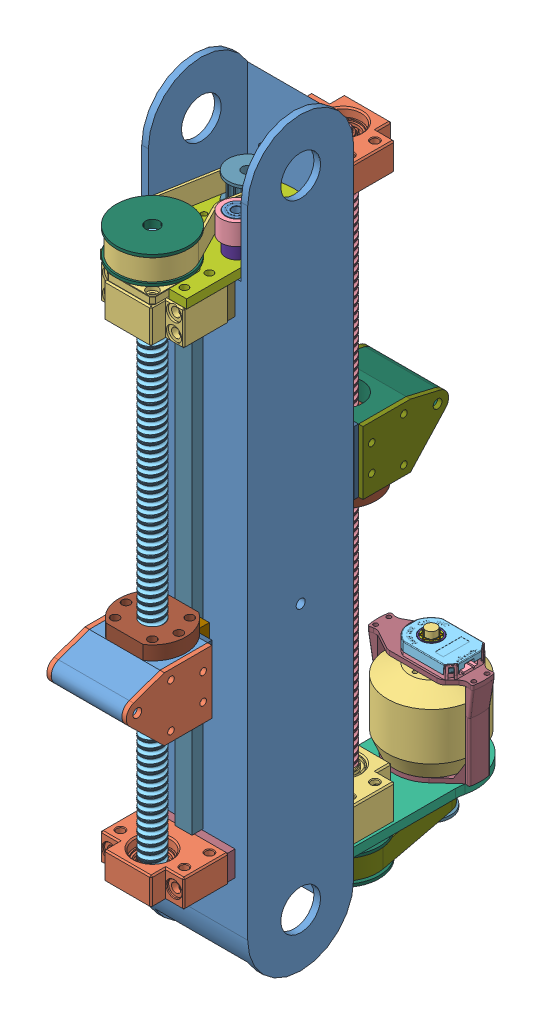
SolidWorks assembly Shoulder, configuration Default. Lengths in mm.
Overall size (98.94 533.4 280.38).
79 component instances, 40 part files, 66 mates.
Components (placement in the parent):
- Box^Shoulder-1: Box^Shoulder [Default] at origin size (76.2 533.4 76.2) (virtual)
- BF12-1: BF12 [Default] at (0 614.1315 -46.7041) x (1 0 0) z (0 1 0) size (60 43 20)
- BK12-1: BK12 [Default] at (0 212.1315 -46.7041) x (-1 0 0) z (0 -1 0) size (60 46.94 35.34)
- SFU1605-450-1: SFU1605-450 [1605-400] at (0 171.1315 -71.7041) x (1 0 0) z (0 -1 0) size (16.52 16.22 450)
- BK12-2: BK12 [Default] at (0 582.269 40.2909) x (-1 0 0) z (0 1 0) size (60 46.94 35.34)
- BF12-2: BF12 [Default] at (0 230.269 40.2909) x (-1 0 0) z (0 1 0) size (60 43 20)
- SFU1605-400-3: SFU1605-400 [1605-400] at (0 623.269 65.2909) x (-1 0 0) z (0 1 0) size (16.52 16.22 400)
- J3Plate^Shoulder-1: J3Plate^Shoulder [Default] at origin size (65 6.35 120.35) (virtual)
- J2Plate^Shoulder-1: J2Plate^Shoulder [Default] at origin size (65 6.35 125.74) (virtual)
- J3MGN12R-1: J3MGN12R [Default] at origin size (12 379.5 8)
- J3MGN12C-1: J3MGN12C [Default] at (0 433.1293 -49.3066) x (1 0 0) z (0 1 0) size (27 10 45.5)
- CarriagePlate^Shoulder-1: CarriagePlate^Shoulder [Default] at (0 67.1524 -3.2066) size (50.8 45.5 3.17) (virtual)
- nut-1: nut [Default] at (0 410.3793 -71.7041) x (-1 0 0) z (0 -1 0) size (48 40 42)
- BKSpacer^Shoulder-1: BKSpacer^Shoulder [Default] at origin size (58 23 5.4) (virtual)
- BKSpacer^Shoulder-2: BKSpacer^Shoulder [Default] at (0 370.1375 81.5975) size (58 23 5.4) (virtual)
- BFSpacer^Shoulder-1: BFSpacer^Shoulder [Default] at origin size (58 18 5.4) (virtual)
- BFSpacer^Shoulder-2: BFSpacer^Shoulder [Default] at (0 -383.8625 81.5975) size (58 18 5.4) (virtual)
- J2MGN12R^Shoulder-1: J2MGN12R^Shoulder [Default] at origin size (12 329.5 8) (virtual)
- J3Adapter^Shoulder-2: J3Adapter^Shoulder [Default] at (0 76.5186 -3.2066) size (57.15 45.79 61.61) (virtual)
  - Body^J3Adapter_Shoulder-1: Body^J3Adapter_Shoulder [Default] at (38.1 26.927 0) x (0 0 -1) z (1 0 0) size (61.61 45.5 50.8) (virtual)
  - SidePlate^J3Adapter_Shoulder-1: SidePlate^J3Adapter_Shoulder [Default] at origin size (3.18 45.5 61.61) (virtual)
  - SidePlate^J3Adapter_Shoulder-2: SidePlate^J3Adapter_Shoulder [Default] at (53.975 0 0) size (3.18 45.5 61.61) (virtual)
  - 94459A340_BRASS HEAT-SET INSERT FOR PLASTIC-1: 94459A340_BRASS HEAT-SET INSERT FOR PLASTIC [94459A340] at (-18.415 340.7357 -83.735) x (0 -1 0) z (0 0 -1) size (7.22 6.55 7.22)
  - 94459A220_BRASS HEAT-SET INSERT FOR PLASTIC-1: 94459A220_BRASS HEAT-SET INSERT FOR PLASTIC [94459A220] at (13.435 346.5607 -81.9325) x (-0.837169 0 -0.546944) z (-0.546944 0 0.837169) size (8.76 13.2 8.76)
- J3MGN12C-2: J3MGN12C [Default] at (0 351.2303 42.8934) x (-1 0 0) z (0 1 0) size (27 10 45.5)
- nut-2: nut [Default] at (0 373.9803 65.2909) x (1 0 0) z (0 1 0) size (48 40 42)
- J2Adapter^Shoulder-1: J2Adapter^Shoulder [Default] at (0 707.841 -3.2066) x (1 0 0) z (0 0 -1) size (57.15 45.79 61.61) (virtual)
  - Body^J2Adapter_Shoulder-1: Body^J2Adapter_Shoulder [Default] at (38.1 26.927 0) x (0 0 -1) z (1 0 0) size (61.61 45.5 50.8) (virtual)
  - SidePlate^J2Adapter_Shoulder-1: SidePlate^J2Adapter_Shoulder [Default] at origin size (3.18 45.5 61.61) (virtual)
  - SidePlate^J2Adapter_Shoulder-2: SidePlate^J2Adapter_Shoulder [Default] at (53.975 0 0) size (3.18 45.5 61.61) (virtual)
  - 94459A340_BRASS HEAT-SET INSERT FOR PLASTIC-1: 94459A340_BRASS HEAT-SET INSERT FOR PLASTIC [94459A340] at (-18.415 340.7357 -83.735) x (0 -1 0) z (0 0 -1) size (7.22 6.55 7.22)
  - 94459A220_BRASS HEAT-SET INSERT FOR PLASTIC-1: 94459A220_BRASS HEAT-SET INSERT FOR PLASTIC [94459A220] at (13.435 346.5607 -81.9325) x (-0.837169 0 -0.546944) z (-0.546944 0 0.837169) size (8.76 13.2 8.76)
- CarriagePlate^Shoulder-2: CarriagePlate^Shoulder [Default] at (0 -14.7465 -3.2066) x (-1 0 0) z (0 0 -1) size (50.8 45.5 3.17) (virtual)
- 192kvMotorEncoded-1: 192kvMotorEncoded [Default] at (0 202.8065 -135.2041) x (0 0 -1) z (1 0 0) size (63 104.52 76.93)
  - BetterKEDA-1: BetterKEDA [Default] at origin size (63 104.52 63)
  - CUI_DEVICES_AMT102-0048-N2000-S-1: CUI_DEVICES_AMT102-0048-N2000-S [Default] at (0 65.12 0) x (1 0 0) z (0 1 0) size (36.33 46.21 9.2)
    - CUI_DEVICES_AMT102-0048-N2000-S.step-1: CUI_DEVICES_AMT102-0048-N2000-S.step [Default] at origin size (36.33 46.21 9.2)
      - AMT-102-Base-REV-K.step-1: AMT-102-Base-REV-K.step [Default] x (-1 0 0) z (0 0 -1) size (28.78 43.39 9.06)
      - AMT-102-Top-Cover-REV-H.step-1: AMT-102-Top-Cover-REV-H.step [Default] at (0 0 5.23) x (-1 0 0) z (0 0 -1) size (28.6 43.26 6.55)
      - AMT-Sleeve-REV-D_ 2 mm.step-1: AMT-Sleeve-REV-D_ 2 mm.step [Default] at (0 0 -2.42) x (0.999996 0.002864 0) z (0 0 1) size (10.79 10.79 7.8)
      - AMT-Hub-Top-REV-D1.step-1: AMT-Hub-Top-REV-D1.step [Default] at (0 0 2.13) x (0.999996 0.002864 0) z (0 0 1) size (14 14 5.67)
      - AMT-Hub-Bottom-REV-B.step-1: AMT-Hub-Bottom-REV-B.step [Default] at (0 0 2.43) x (0.999998 -0.001942 0) z (0 0 1) size (17.3 17.3 3.2)
      - AMT10X-Shaft-Adaptor-REV-E.step-1: AMT10X-Shaft-Adaptor-REV-E.step [Default] at (0 0 0.03) x (0.999996 0.002864 0) z (0 0 1) size (11.8 11.8 7.8)
      - Receiver-board.step-1: Receiver-board.step [Default] at (72.2834 -20.351 3.03) x (-1 0 0) z (0 0 -1) size (26.5 26.62 0.41)
      - Rotor-board-REV F.step-1: Rotor-board-REV F.step [Default] at (0 0 2.13) x (0.807874 -0.589355 0) z (0 0 1) size (26 26 0.3)
      - Transmitter-board AMT10_AMT-102.step-1: Transmitter-board AMT10_AMT-102.step [Default] at (19.1596 -17.1102 1.22) x (-1 0 0) z (0 0 -1) size (26.63 38.43 4.41)
  - Body^192kvMotorEncoded-1: Body^192kvMotorEncoded [Default] at origin size (53 64.53 76.93) (virtual)
- 192kvMotorEncoded-2: 192kvMotorEncoded [Default] at (0 591.594 -3.2066) x (-0.707107 0 -0.707107) z (-0.707107 0 0.707107) size (63 104.52 76.93)
  - BetterKEDA-1: BetterKEDA [Default] at origin size (63 104.52 63)
  - CUI_DEVICES_AMT102-0048-N2000-S-1: CUI_DEVICES_AMT102-0048-N2000-S [Default] at (0 65.12 0) x (1 0 0) z (0 1 0) size (36.33 46.21 9.2)
    - CUI_DEVICES_AMT102-0048-N2000-S.step-1: CUI_DEVICES_AMT102-0048-N2000-S.step [Default] at origin size (36.33 46.21 9.2)
      - AMT-102-Base-REV-K.step-1: AMT-102-Base-REV-K.step [Default] x (-1 0 0) z (0 0 -1) size (28.78 43.39 9.06)
      - AMT-102-Top-Cover-REV-H.step-1: AMT-102-Top-Cover-REV-H.step [Default] at (0 0 5.23) x (-1 0 0) z (0 0 -1) size (28.6 43.26 6.55)
      - AMT-Sleeve-REV-D_ 2 mm.step-1: AMT-Sleeve-REV-D_ 2 mm.step [Default] at (0 0 -2.42) x (0.999996 0.002864 0) z (0 0 1) size (10.79 10.79 7.8)
      - AMT-Hub-Top-REV-D1.step-1: AMT-Hub-Top-REV-D1.step [Default] at (0 0 2.13) x (0.999996 0.002864 0) z (0 0 1) size (14 14 5.67)
      - AMT-Hub-Bottom-REV-B.step-1: AMT-Hub-Bottom-REV-B.step [Default] at (0 0 2.43) x (0.999998 -0.001942 0) z (0 0 1) size (17.3 17.3 3.2)
      - AMT10X-Shaft-Adaptor-REV-E.step-1: AMT10X-Shaft-Adaptor-REV-E.step [Default] at (0 0 0.03) x (0.999996 0.002864 0) z (0 0 1) size (11.8 11.8 7.8)
      - Receiver-board.step-1: Receiver-board.step [Default] at (72.2834 -20.351 3.03) x (-1 0 0) z (0 0 -1) size (26.5 26.62 0.41)
      - Rotor-board-REV F.step-1: Rotor-board-REV F.step [Default] at (0 0 2.13) x (0.807874 -0.589355 0) z (0 0 1) size (26 26 0.3)
      - Transmitter-board AMT10_AMT-102.step-1: Transmitter-board AMT10_AMT-102.step [Default] at (19.1596 -17.1102 1.22) x (-1 0 0) z (0 0 -1) size (26.63 38.43 4.41)
  - Body^192kvMotorEncoded-1: Body^192kvMotorEncoded [Default] at origin size (53 64.53 76.93) (virtual)
- 15Tpulley-3: 15Tpulley [Default] at (0 175.8815 -135.2041) size (28 28 28)
- 15Tpulley-4: 15Tpulley [Default] at (0 618.519 -3.2066) x (-1 0 0) z (0 0 1) size (28 28 28)
- 30Tpulley-3: 30Tpulley [Default] at (0 618.519 65.2909) size (52 20 52)
- 30Tpulley-4: 30Tpulley [Default] at (0 175.8815 -71.7041) size (52 20 52)
- J3Belt^Shoulder-1: J3Belt^Shoulder [Default] at origin size (49.49 15 101.05) (virtual)
- TensionPillarJ3-1: TensionPillarJ3 [Default] at (-42.5291 257.8915 3.8215) size (22.22 25.73 22.23)
  - 92510A774_ALUM UNTHRD SPACER-1-1: 92510A774_ALUM UNTHRD SPACER-1 [92510A774] at (20.3041 -69.3725 -110.4505) x (1 0 0) z (0 1 0) size (15.88 15.88 9.53)
  - 98019A228_MIL SPEC. 300 SERIES SS FLAT WASHER-1: 98019A228_MIL SPEC. 300 SERIES SS FLAT WASHER [98019A228] at (20.3041 -74.8462 -110.4505) x (0.972939 0 -0.231063) z (0.231063 0 0.972939) size (9.53 0.71 9.53)
  - 60355K701_BALL BEARING-1: 60355K701_BALL BEARING [60355K701] at (20.3041 -77.3354 -110.4505) x (1 0 0) z (0 1 0) size (15.88 15.88 4.98)
  - Roller^TensionPillarJ3-1: Roller^TensionPillarJ3 [Default] at (20.3041 -17.1652 2.6827) size (22.23 15 22.23) (virtual)
  - 60355K701_BALL BEARING-2: 60355K701_BALL BEARING [60355K701] at (20.3041 -87.8548 -110.4505) x (1 0 0) z (0 1 0) size (15.88 15.88 4.98)
- J2Belt^Shoulder-1: J2Belt^Shoulder [Default] at origin size (49.49 15 106.05) (virtual)
- TensionPillarJ2-1: TensionPillarJ2 [Default] at (-24.3623 536.509 127.3519) x (-0.837169 0 -0.546944) z (-0.546944 0 0.837169) size (22.22 25.73 22.23)
  - 92510A774_ALUM UNTHRD SPACER-1-1: 92510A774_ALUM UNTHRD SPACER-1 [92510A774] at (20.3041 -69.3725 -110.4505) x (1 0 0) z (0 1 0) size (15.88 15.88 9.53)
  - 98019A228_MIL SPEC. 300 SERIES SS FLAT WASHER-1: 98019A228_MIL SPEC. 300 SERIES SS FLAT WASHER [98019A228] at (20.3041 -74.8462 -110.4505) x (0.972939 0 -0.231063) z (0.231063 0 0.972939) size (9.53 0.71 9.53)
  - 60355K701_BALL BEARING-1: 60355K701_BALL BEARING [60355K701] at (20.3041 -77.3354 -110.4505) x (1 0 0) z (0 1 0) size (15.88 15.88 4.98)
  - Roller^TensionPillarJ2-1: Roller^TensionPillarJ2 [Default] at (20.3041 -17.1652 2.6827) size (22.23 15 22.23) (virtual)
  - 60355K701_BALL BEARING-2: 60355K701_BALL BEARING [60355K701] at (20.3041 -87.8548 -110.4505) x (1 0 0) z (0 1 0) size (15.88 15.88 4.98)
Mates (geometry in assembly coordinates):
- Parallel1: parallel anti-aligned: plane of Box^Shoulder-1 through (-33.3375 186.9315 -41.3066) normal (0 0 -1); plane of BF12-1 through (29 605.1315 -46.7041) normal (0 0 1)
- Width1: width anti-aligned: plane of BF12-1 through (30 605.1315 -78.2041) normal (1 0 0); plane of Box^Shoulder-1 through (-30 605.1315 -47.7041) normal (-1 0 0); plane of BF12-1 through (38.1 644.1315 -3.2066) normal (1 0 0); plane of Box^Shoulder-1 through (-38.1 186.9315 -3.2066) normal (-1 0 0)
- Distance6: distance anti-aligned: plane of Box^Shoulder-1 through (-33.3375 186.9315 -41.3066) normal (0 0 -1); plane of BK12-1 through (-29 223.6315 -46.7041) normal (0 0 1)
- Width2: width aligned: plane of BK12-1 through (30 223.6315 -47.7041) normal (1 0 0); plane of Box^Shoulder-1 through (-30 223.6315 -78.2041) normal (-1 0 0); plane of BK12-1 through (-38.1 186.9315 -3.2066) normal (-1 0 0); plane of Box^Shoulder-1 through (38.1 644.1315 -3.2066) normal (1 0 0)
- Parallel3: parallel aligned: plane of BK12-1 through (29 224.6315 -47.7041) normal (0 1 0)
- Coincident11: coincident: line of SFU1605-450-1 through (0 185.8815 -71.7041) axis (0 -1 0)
- Concentric6: concentric anti-aligned: cylinder of BK12-1 through (0 220.1315 -71.7041) axis (0 1 0) radius 6; cylinder of SFU1605-450-1 through (0 186.1315 -71.7041) axis (0 -1 0) radius 5
- Coincident12: coincident anti-aligned: plane of BK12-1 through (7.2358 225.1315 -64.4683) normal (0 1 0); plane of SFU1605-450-1 through (0 225.1315 -71.7041) normal (0 -1 0)
- Coincident13: coincident anti-aligned: plane of BF12-1 through (-6.5021 610.1315 -65.202) normal (0 -1 0); plane of SFU1605-450-1 through (0 610.1315 -71.7041) normal (0 1 0)
- Distance3: distance = 12.7 mm: plane of BK12-1 through (29 199.6315 -47.7041) normal (0 -1 0); line of Box^Shoulder-1 through (38.1 186.9315 -41.3066) axis (-1 0 0)
- Coincident27: coincident: line of SFU1605-400-3 through (0 608.519 65.2909) axis (0 1 0)
- Concentric18: concentric anti-aligned: cylinder of BK12-2 through (0 582.269 65.2909) axis (0 -1 0) radius 6; cylinder of SFU1605-400-3 through (0 608.269 65.2909) axis (0 1 0) radius 5
- Distance8: distance anti-aligned: plane of Box^Shoulder-1 through (-33.3375 186.9315 34.8934) normal (0 0 1); plane of BK12-2 through (-29 570.769 40.2909) normal (0 0 -1)
- Coincident29: coincident anti-aligned: plane of BK12-2 through (7.2358 569.269 58.0551) normal (0 -1 0); plane of SFU1605-400-3 through (0 569.269 65.2909) normal (0 1 0)
- Coincident30: coincident anti-aligned: plane of BF12-2 through (-6.5021 234.269 58.7888) normal (0 1 0); plane of SFU1605-400-3 through (0 234.269 65.2909) normal (0 -1 0)
- Concentric19: concentric anti-aligned: cylinder of BF12-2 through (0 227.069 65.2909) axis (0 1 0) radius 5; cylinder of SFU1605-400-3 through (0 234.269 65.2909) axis (0 -1 0) radius 5
- Distance5: distance = 33.3375 mm: line of Box^Shoulder-1 through (38.1 186.9315 34.8934) axis (-1 0 0); plane of BF12-2 through (29 220.269 41.2909) normal (0 -1 0)
- Coincident35: coincident anti-aligned: plane of J3MGN12R-1 through (0 0 -49.3066) normal (0 0 -1); plane of J3MGN12C-1 through (-6 455.8793 -49.3066) normal (0 0 1)
- Width3: width anti-aligned: plane of J3MGN12C-1 through (13.5 455.8793 -44.3066) normal (1 0 0); plane of J3MGN12C-1 through (-13.5 455.8793 -44.3066) normal (-1 0 0); plane of J3MGN12R-1 through (-6 604.1315 -49.3066) normal (-1 0 0); plane of J3MGN12R-1 through (6 604.1315 -49.3066) normal (1 0 0)
- Coincident36: coincident anti-aligned: plane of J3MGN12C-1 through (13.5 455.8793 -54.3066) normal (0 0 -1); plane of CarriagePlate^Shoulder-1 through (0 67.1524 -54.3066) normal (0 0 1)
- Concentric22: concentric anti-aligned: cylinder of J3MGN12C-1 through (10 443.1293 -50.3066) axis (0 0 -1) radius 1.5; cylinder of CarriagePlate^Shoulder-1 through (10 443.1293 -57.4816) axis (0 0 1) radius 1.5
- Concentric23: concentric anti-aligned: cylinder of J3MGN12C-1 through (-10 423.1293 -50.3066) axis (0 0 -1) radius 1.5; cylinder of CarriagePlate^Shoulder-1 through (-10 423.1293 -57.4816) axis (0 0 1) radius 1.5
- Concentric24: concentric aligned: cylinder of SFU1605-450-1 through (0 610.1315 -71.7041) axis (0 1 0) radius 5; cylinder of nut-1 through (0 400.3793 -71.7041) axis (0 1 0) radius 8
- Concentric25: concentric aligned: cylinder of BF12-1 through (0 610.9315 -71.7041) axis (0 1 0) radius 5; cylinder of SFU1605-450-1 through (0 610.1315 -71.7041) axis (0 1 0) radius 5
- Coincident37: coincident anti-aligned: plane of CarriagePlate^Shoulder-1 through (-25.4 410.3793 -57.4816) normal (0 -1 0); plane of nut-1 through (0 410.3793 -71.7041) normal (0 1 0)
- Parallel4: parallel anti-aligned: plane of Box^Shoulder-1 through (-33.3375 186.9315 34.8934) normal (0 0 1); plane of BF12-2 through (-29 221.269 40.2909) normal (0 0 -1)
- Concentric27: concentric anti-aligned: cylinder of BK12-2 through (-23 575.769 40.2909) axis (0 0 1) radius 3.3; cylinder of BKSpacer^Shoulder-2 through (-23 575.769 102.6848) axis (0 0 -1) radius 3.3
- Concentric28: concentric anti-aligned: cylinder of BK12-2 through (23 575.769 40.2909) axis (0 0 1) radius 3.3; cylinder of BKSpacer^Shoulder-2 through (23 575.769 102.6848) axis (0 0 -1) radius 3.3
- Coincident42: coincident anti-aligned: plane of Box^Shoulder-1 through (-33.3375 186.9315 34.8934) normal (0 0 1); plane of BKSpacer^Shoulder-2 through (0 370.1375 34.8934) normal (0 0 -1)
- Concentric29: concentric anti-aligned: cylinder of BF12-2 through (23 230.269 40.2909) axis (0 0 1) radius 3.3; cylinder of BFSpacer^Shoulder-2 through (23 230.269 101.0198) axis (0 0 -1) radius 3.3
- Concentric30: concentric anti-aligned: cylinder of BF12-2 through (-23 230.269 40.2909) axis (0 0 1) radius 3.3; cylinder of BFSpacer^Shoulder-2 through (-23 230.269 101.0198) axis (0 0 -1) radius 3.3
- Coincident43: coincident anti-aligned: plane of Box^Shoulder-1 through (-33.3375 186.9315 34.8934) normal (0 0 1); plane of BFSpacer^Shoulder-2 through (0 -383.8625 34.8934) normal (0 0 -1)
- Concentric32: concentric anti-aligned: cylinder of nut-1 through (0 442.3793 -71.7041) axis (0 -1 0) radius 14; cylinder of Adapter^Shoulder-2/Body^Adapter_Shoulder-1 through (0 349.1272 -71.7041) axis (0 1 0) radius 14
- Parallel6: parallel anti-aligned: plane of CarriagePlate^Shoulder-1 through (0 67.1524 -57.4816) normal (0 0 -1); plane of Adapter^Shoulder-2/Body^Adapter_Shoulder-1 through (38.1 349.1272 -57.4816) normal (0 0 1)
- Coincident47: coincident anti-aligned: plane of nut-1 through (0 410.3793 -71.7041) normal (0 1 0); plane of Adapter^Shoulder-2/Body^Adapter_Shoulder-1 through (-25.4 410.3793 -57.4816) normal (0 -1 0)
- Coincident48: coincident anti-aligned: plane of nut-1 through (0 410.3793 -71.7041) normal (0 1 0); plane of Adapter^Shoulder-2/Body^Adapter_Shoulder-1 through (-25.4 410.3793 -57.4816) normal (0 -1 0)
- Coincident49: coincident anti-aligned: plane of nut-1 through (0 410.3793 -71.7041) normal (0 1 0); plane of Adapter^Shoulder-2/Body^Adapter_Shoulder-1 through (-25.4 410.3793 -57.4816) normal (0 -1 0)
- Coincident51: coincident anti-aligned: plane of J2MGN12R^Shoulder-1 through (0 0 42.8934) normal (0 0 1); plane of J3MGN12C-2 through (6 373.9803 42.8934) normal (0 0 -1)
- Width6: width anti-aligned: plane of J3MGN12C-2 through (-13.5 373.9803 37.8934) normal (-1 0 0); plane of J3MGN12C-2 through (13.5 373.9803 37.8934) normal (1 0 0); plane of J2MGN12R^Shoulder-1 through (6 569.769 42.8934) normal (1 0 0); plane of J2MGN12R^Shoulder-1 through (-6 569.769 42.8934) normal (-1 0 0)
- Concentric34: concentric anti-aligned: cylinder of SFU1605-400-3 through (0 608.269 65.2909) axis (0 1 0) radius 5; cylinder of nut-2 through (0 383.9803 65.2909) axis (0 -1 0) radius 8
- Coincident52: coincident anti-aligned: plane of J3MGN12C-2 through (0 373.9803 42.8934) normal (0 1 0); plane of nut-2 through (0 373.9803 65.2909) normal (0 -1 0)
- Concentric35: concentric anti-aligned: cylinder of nut-2 through (0 341.9803 65.2909) axis (0 1 0) radius 14; cylinder of J2Adapter^Shoulder-1/Body^J2Adapter_Shoulder-1 through (0 435.2324 65.2909) axis (0 -1 0) radius 14
- Parallel7: parallel anti-aligned: plane of J3MGN12C-2 through (-13.5 373.9803 47.8934) normal (0 0 1); plane of J2Adapter^Shoulder-1/Body^J2Adapter_Shoulder-1 through (38.1 435.2324 51.0684) normal (0 0 -1)
- Coincident54: coincident anti-aligned: plane of nut-2 through (0 373.9803 65.2909) normal (0 -1 0); plane of J2Adapter^Shoulder-1/Body^J2Adapter_Shoulder-1 through (-25.4 373.9803 51.0684) normal (0 1 0)
- Concentric36: concentric anti-aligned: cylinder of J3MGN12C-2 through (10 361.2303 43.8934) axis (0 0 1) radius 1.5; cylinder of CarriagePlate^Shoulder-2 through (10 361.2303 51.0684) axis (0 0 -1) radius 1.5
- Concentric37: concentric anti-aligned: cylinder of J3MGN12C-2 through (-10 341.2303 43.8934) axis (0 0 1) radius 1.5; cylinder of CarriagePlate^Shoulder-2 through (-10 341.2303 51.0684) axis (0 0 -1) radius 1.5
- Coincident55: coincident anti-aligned: plane of J3MGN12C-2 through (-13.5 373.9803 47.8934) normal (0 0 1); plane of CarriagePlate^Shoulder-2 through (0 -14.7465 47.8934) normal (0 0 -1)
- Parallel8: parallel aligned: plane of BF12-2 through (29 240.269 41.2909) normal (0 1 0)
- Concentric38: concentric aligned: cylinder of J3Plate^Shoulder-1 through (0 193.2815 -135.2041) axis (0 1 0) radius 15.875; cylinder of 192kvMotorEncoded-1/BetterKEDA-1 through (0 173.2815 -135.2041) axis (0 1 0) radius 4
- Concentric39: concentric aligned: cylinder of J3Plate^Shoulder-1 through (0 193.2815 -113.0041) axis (0 1 0) radius 2; cylinder of 192kvMotorEncoded-1/Body^192kvMotorEncoded-1 through (0 199.6315 -113.0041) axis (0 1 0) radius 2
- Coincident56: coincident anti-aligned: plane of J3Plate^Shoulder-1 through (56.3375 199.6315 -121.8438) normal (0 1 0); plane of 192kvMotorEncoded-1/Body^192kvMotorEncoded-1 through (0 199.6315 -135.2041) normal (0 -1 0)
- Concentric40: concentric aligned: cylinder of J2Plate^Shoulder-1 through (0 601.119 -3.2066) axis (0 -1 0) radius 15.875; cylinder of 192kvMotorEncoded-2/BetterKEDA-1 through (0 621.119 -3.2066) axis (0 -1 0) radius 4
- Concentric41: concentric aligned: cylinder of J2Plate^Shoulder-1 through (-15.6978 601.119 12.4912) axis (0 -1 0) radius 2; cylinder of 192kvMotorEncoded-2/Body^192kvMotorEncoded-1 through (-15.6978 594.769 12.4912) axis (0 -1 0) radius 2
- Coincident57: coincident anti-aligned: plane of J2Plate^Shoulder-1 through (0 594.769 0) normal (0 -1 0); plane of 192kvMotorEncoded-2/Body^192kvMotorEncoded-1 through (0 594.769 -3.2066) normal (0 1 0)
- Concentric42: concentric anti-aligned: cylinder of 192kvMotorEncoded-1/BetterKEDA-1 through (0 173.2815 -135.2041) axis (0 1 0) radius 4; cylinder of 15Tpulley-3 through (0 183.8815 -135.2041) axis (0 -1 0) radius 4
- Concentric44: concentric anti-aligned: cylinder of 192kvMotorEncoded-2/BetterKEDA-1 through (0 621.119 -3.2066) axis (0 -1 0) radius 4; cylinder of 15Tpulley-4 through (0 610.519 -3.2066) axis (0 1 0) radius 4
- Concentric45: concentric anti-aligned: cylinder of SFU1605-400-3 through (0 608.269 65.2909) axis (0 1 0) radius 5; cylinder of 30Tpulley-3 through (0 626.519 65.2909) axis (0 -1 0) radius 5
- Coincident61: coincident anti-aligned: circle of SFU1605-400-3; plane of 30Tpulley-3 through (0 608.519 65.2909) normal (0 -1 0)
- Coincident62: coincident aligned: plane of 15Tpulley-4 through (0 626.519 -3.2066) normal (0 -1 0); plane of 30Tpulley-3 through (0 626.519 65.2909) normal (0 -1 0)
- Concentric47: concentric aligned: cylinder of SFU1605-450-1 through (0 186.1315 -71.7041) axis (0 -1 0) radius 5; cylinder of 30Tpulley-4 through (0 183.8815 -71.7041) axis (0 -1 0) radius 5
- Coincident63: coincident anti-aligned: circle of SFU1605-450-1; plane of 30Tpulley-4 through (0 185.8815 -71.7041) normal (0 1 0)
- Coincident64: coincident aligned: plane of 15Tpulley-3 through (0 167.8815 -135.2041) normal (0 1 0); plane of 30Tpulley-4 through (0 167.8815 -71.7041) normal (0 1 0)
- Concentric48: concentric aligned: cylinder of J3Plate^Shoulder-1 through (-22.225 199.6315 -106.6291) axis (0 -1 0) radius 3.175; cylinder of TensionPillarJ3-1/92510A774_ALUM UNTHRD SPACER-1-1 through (-22.225 193.2815 -106.6291) axis (0 -1 0) radius 3.2004
- Coincident65: coincident anti-aligned: plane of J3Plate^Shoulder-1 through (56.3375 193.2815 -121.8438) normal (0 -1 0); plane of TensionPillarJ3-1/92510A774_ALUM UNTHRD SPACER-1-1 through (-22.225 193.2815 -106.6291) normal (0 1 0)
- Concentric49: concentric aligned: cylinder of J2Plate^Shoulder-1 through (19.05 587.4052 23.7809) axis (0 1 0) radius 2.6035; cylinder of TensionPillarJ2-1/92510A774_ALUM UNTHRD SPACER-1-1 through (19.05 601.119 23.7809) axis (0 1 0) radius 3.2004
- Coincident66: coincident anti-aligned: plane of J2Plate^Shoulder-1 through (0 601.119 0) normal (0 1 0); plane of TensionPillarJ2-1/92510A774_ALUM UNTHRD SPACER-1-1 through (19.05 601.119 23.7809) normal (0 -1 0)
